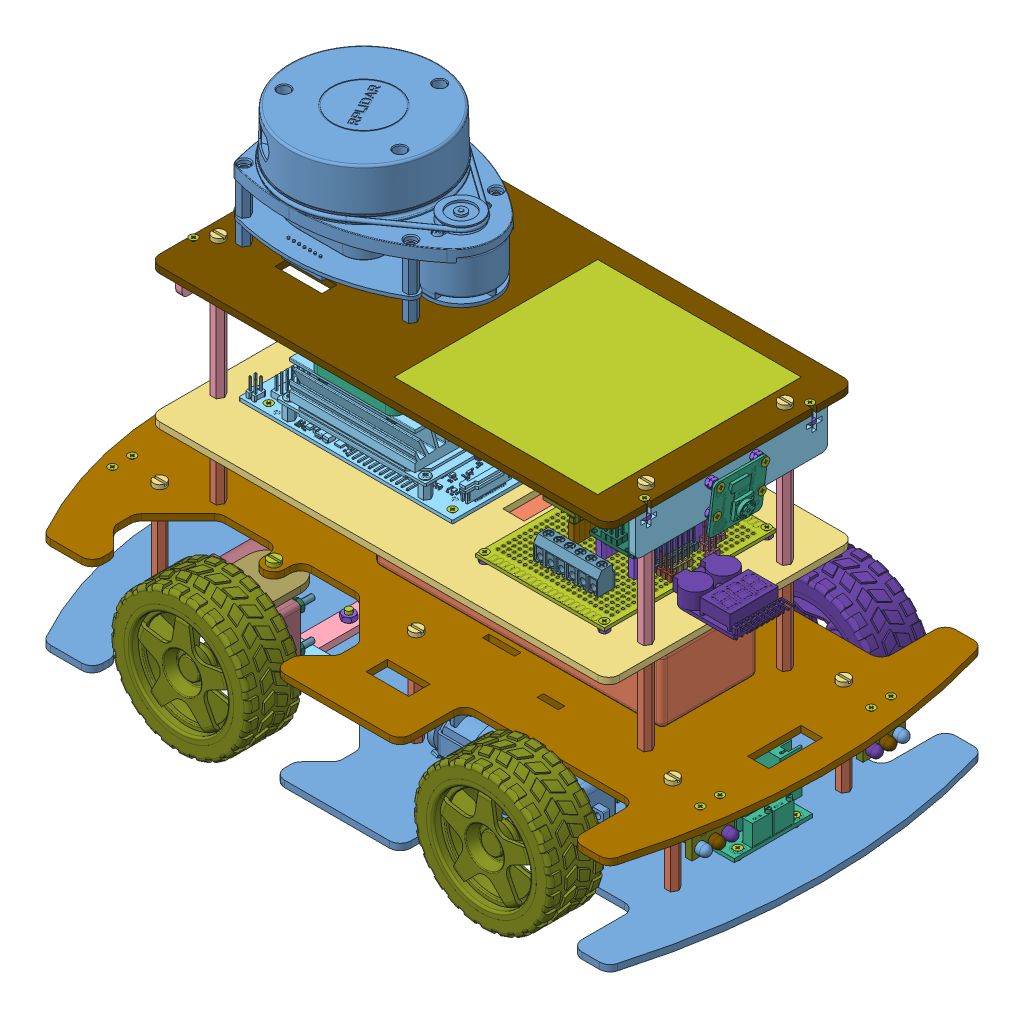
SolidWorks assembly Nigel - Motion Analysis, configuration Default. Lengths in mm.
Overall size (300 217.1 179.17).
273 component instances, 61 part files, 576 mates.
Components (placement in the parent):
- Platform 1-1: Platform 1 [Default] at origin size (300 3 175)
- M3x40 F-F Standoff-1: M3x40 F-F Standoff [Default] at (-1.4467 -726.2923 -120.9176) size (5.77 40 5)
- M3x40 F-F Standoff-2: M3x40 F-F Standoff [Default] at (-1.4467 -726.2923 -200.9176) size (5.77 40 5)
- M3x40 F-F Standoff-3: M3x40 F-F Standoff [Default] at (118.5533 -726.2923 -120.9176) size (5.77 40 5)
- M3x40 F-F Standoff-4: M3x40 F-F Standoff [Default] at (118.5533 -726.2923 -200.9176) size (5.77 40 5)
- M3x40 F-F Standoff-5: M3x40 F-F Standoff [Default] at (238.5533 -726.2923 -120.9176) size (5.77 40 5)
- M3x40 F-F Standoff-6: M3x40 F-F Standoff [Default] at (238.5533 -726.2923 -200.9176) size (5.77 40 5)
- M3x8 Bolt-1: M3x8 Bolt [Default] at (-120 0 40) x (1 0 0) z (0 0 -1) size (5.7 10 5.7)
- M3x8 Bolt-2: M3x8 Bolt [Default] at (-120 0 -40) x (1 0 0) z (0 0 -1) size (5.7 10 5.7)
- M3x8 Bolt-3: M3x8 Bolt [Default] at (0 0 40) x (1 0 0) z (0 0 -1) size (5.7 10 5.7)
- M3x8 Bolt-4: M3x8 Bolt [Default] at (0 0 -40) x (1 0 0) z (0 0 -1) size (5.7 10 5.7)
- M3x8 Bolt-5: M3x8 Bolt [Default] at (120 0 40) x (1 0 0) z (0 0 -1) size (5.7 10 5.7)
- M3x8 Bolt-6: M3x8 Bolt [Default] at (120 0 -40) x (1 0 0) z (0 0 -1) size (5.7 10 5.7)
- Steering Link 1-2: Steering Link 1 [Default] at (-61.537 3 0) x (0 0 1) z (-1 0 0) size (100 3 10)
- Steering Knuckle 1-1: Steering Knuckle 1 [Default] at (-61.537 6 0) x (0 0 -1) z (1 0 0) size (32.95 3 42.5)
- Steering Knuckle 1-2: Steering Knuckle 1 [Default] at (-61.537 9 0) x (0 0 1) z (1 0 0) size (32.95 3 42.5)
- Steering Link 2-2: Steering Link 2 [Default] at (-11.537 9 0) x (0 0 1) z (-1 0 0) size (84.1 3 10)
- M3x10 Bolt-1: M3x10 Bolt [Default] at (-61.537 0 -10) x (1 0 0) z (0 0 -1) size (5.7 12 5.7)
- M3 Nut-2: M3 Nut [Default] at (-61.537 6 -10) size (5.5 2.4 6.98)
- M3x10 Bolt-2: M3x10 Bolt [Default] at (-61.537 0 10) x (1 0 0) z (0 0 -1) size (5.7 12 5.7)
- M3 Nut-3: M3 Nut [Default] at (-61.537 6 10) size (5.5 2.4 6.98)
- M3x14 Bolt-1: M3x14 Bolt [Default] at (-61.537 9 45) size (5.7 16 5.7)
- M3 Nut-4: M3 Nut [Default] at (-61.537 -2.6 45) size (5.5 2.4 6.98)
- M3x14 Bolt-2: M3x14 Bolt [Default] at (-61.537 9 -45) size (5.7 16 5.7)
- M3 Nut-5: M3 Nut [Default] at (-61.537 -2.6 -45) size (5.5 2.4 6.98)
- M3x10 Bolt-3: M3x10 Bolt [Default] at (-36.537 5.8 37.0517) x (1 0 0) z (0 0 -1) size (5.7 12 5.7)
- M3 Nut-6: M3 Nut [Default] at (-36.537 12 37.0517) size (5.5 2.4 6.98)
- M3x10 Bolt-4: M3x10 Bolt [Default] at (-36.537 5.8 -37.0517) x (1 0 0) z (0 0 -1) size (5.7 12 5.7)
- M3 Nut-7: M3 Nut [Default] at (-36.537 12 -37.0517) size (5.5 2.4 6.98)
- M3x25 Bolt-1: M3x25 Bolt [Default] at (-36.537 9 0) x (1 0 0) z (0 0 -1) size (5.7 27 5.7)
- M3 Nut-1: M3 Nut [Default] at (-36.537 12 0) size (5.5 2.4 6.98)
- M3 Nut-14: M3 Nut [Default] at (-36.537 25.75 0) size (5.5 2.4 6.98)
- Front Motor Mount-1: Front Motor Mount [Default] at (-61.537 23 -60.5) x (1 0 0) z (0 0 -1) size (25 37 3)
- Front Motor Mount-2: Front Motor Mount [Default] at (-61.537 23 57.5) x (1 0 0) z (0 0 -1) size (25 37 3)
- Steering Knuckle 2-1: Steering Knuckle 2 [Default] at (-61.537 40 50) x (0 0 -1) z (1 0 0) size (30 3 25)
- Steering Knuckle 2-2: Steering Knuckle 2 [Default] at (-61.537 40 -50) x (0 0 1) z (-1 0 0) size (30 3 25)
- Front Wheel Hub-1: Front Wheel Hub [Default] at (-71.9938 11.75 35.7704) x (0 0 -1) z (1 0 0) size (40.5 22.5 47)
- M2.5x25 Bolt-1: M2.5x25 Bolt [Default] at (-53.037 31.75 60.5) x (1 0 0) z (0 -1 0) size (5.1 27 5.1)
- M2.5 Nut-1: M2.5 Nut [Default] at (-53.037 31.75 41.5) x (1 0 0) z (0 -1 0) size (5 2 6.35)
- M2.5x25 Bolt-2: M2.5x25 Bolt [Default] at (-53.037 14.25 60.5) x (1 0 0) z (0 -1 0) size (5.1 27 5.1)
- M2.5 Nut-2: M2.5 Nut [Default] at (-53.037 14.25 41.5) x (1 0 0) z (0 -1 0) size (5 2 6.35)
- Front Wheel Hub-2: Front Wheel Hub [Default] at (-71.9938 34.25 -35.7704) x (0 0 1) z (1 0 0) size (40.5 22.5 47)
- M2.5x25 Bolt-3: M2.5x25 Bolt [Default] at (-53.037 31.75 -60.5) x (1 0 0) z (0 1 0) size (5.1 27 5.1)
- M2.5 Nut-3: M2.5 Nut [Default] at (-53.037 31.75 -43.5) x (1 0 0) z (0 -1 0) size (5 2 6.35)
- M2.5x25 Bolt-4: M2.5x25 Bolt [Default] at (-53.037 14.25 -60.5) x (1 0 0) z (0 1 0) size (5.1 27 5.1)
- M2.5 Nut-4: M2.5 Nut [Default] at (-53.037 14.25 -43.5) x (1 0 0) z (0 -1 0) size (5 2 6.35)
- Left Wheel-1: Left Wheel [Default] at (-79.9477 -3.5128 34.4259) size (65 65 30.09)
- Right Wheel-1: Right Wheel [Default] at (-48.2819 2.8225 -42.4013) x (-1 0 0) z (0 0 -1) size (65 65 30.09)
- Rear Motor Mount-1: Rear Motor Mount [Default] at (59.4 23 -37.9) size (25 46 3)
- Rear Motor Mount-2: Rear Motor Mount [Default] at (59.4 23 34.9) size (25 46 3)
- Rear Motor-1: Rear Motor [Default] at (119.5998 48.0831 -84.1205) x (0 -1 0) z (-1 0 0) size (29.86 44.39 75.48)
- Rear Motor-2: Rear Motor [Default] at (119.5998 -2.0831 84.1205) x (0 1 0) z (-1 0 0) size (29.86 44.39 75.48)
- M3x25 Bolt-2: M3x25 Bolt [Default] at (59.4 31.75 56.5) x (1 0 0) z (0 -1 0) size (5.7 27 5.7)
- M3 Nut-10: M3 Nut [Default] at (59.4 31.75 32.5) x (1 0 0) z (0 -1 0) size (5.5 2.4 6.98)
- M3x25 Bolt-3: M3x25 Bolt [Default] at (59.4 14.25 56.5) x (1 0 0) z (0 -1 0) size (5.7 27 5.7)
- M3 Nut-11: M3 Nut [Default] at (59.4 14.25 32.5) x (1 0 0) z (0 -1 0) size (5.5 2.4 6.98)
- M3x25 Bolt-4: M3x25 Bolt [Default] at (59.4 31.75 -56.5) x (1 0 0) z (0 1 0) size (5.7 27 5.7)
- M3 Nut-12: M3 Nut [Default] at (59.4 31.75 -34.9) x (1 0 0) z (0 -1 0) size (5.5 2.4 6.98)
- M3x25 Bolt-5: M3x25 Bolt [Default] at (59.4 14.25 -56.5) x (1 0 0) z (0 1 0) size (5.7 27 5.7)
- M3 Nut-13: M3 Nut [Default] at (59.4 14.25 -34.9) x (1 0 0) z (0 -1 0) size (5.5 2.4 6.98)
- Left Wheel-2: Left Wheel [Default] at (61.5893 -3.6128 34.4259) size (65 65 30.09)
- Right Wheel-2: Right Wheel [Default] at (93.2551 2.9225 -42.4013) x (-1 0 0) z (0 0 -1) size (65 65 30.09)
- Motor Driver-1: Motor Driver [Default] at (32.2636 -15.779 -17.5479) x (0 0 1) z (-1 0 0) size (49.64 15.8 28)
- M4x5 Spacer-1: M4x5 Spacer [Default] at (-15 3 21) size (7 5 7)
- M4x5 Spacer-2: M4x5 Spacer [Default] at (-15 3 -21) size (7 5 7)
- M4x5 Spacer-3: M4x5 Spacer [Default] at (9 3 21) size (7 5 7)
- M4x5 Spacer-4: M4x5 Spacer [Default] at (9 3 -21) size (7 5 7)
- M3x14 Bolt-3: M3x14 Bolt [Default] at (-15 9.5 21) size (5.7 16 5.7)
- M3 Nut-15: M3 Nut [Default] at (-15 -2.4 21) size (5.5 2.4 6.98)
- M3x14 Bolt-4: M3x14 Bolt [Default] at (-15 9.5 -21) size (5.7 16 5.7)
- M3 Nut-16: M3 Nut [Default] at (-15 -2.4 -21) size (5.5 2.4 6.98)
- M3x14 Bolt-5: M3x14 Bolt [Default] at (9 9.5 21) size (5.7 16 5.7)
- M3 Nut-17: M3 Nut [Default] at (9 -2.4 21) size (5.5 2.4 6.98)
- M3x14 Bolt-6: M3x14 Bolt [Default] at (9 9.5 -21) size (5.7 16 5.7)
- M3 Nut-18: M3 Nut [Default] at (9 -2.4 -21) size (5.5 2.4 6.98)
- M12 Push Button-1: M12 Push Button [Default] at (36 0 0) x (1 0 0) z (0 -1 0) size (15.74 16.08 24.73)
- M12 Push Button Nut-1: M12 Push Button Nut [Default] at (36 -0.5 0) x (1 0 0) z (0 -1 0) size (15.79 14.76 2.3)
- Buck Converter-2: Buck Converter [Default] at (94.4 5.5 0) size (65.3 28.6 46.4)
- M2x10 Bolt-5: M2x10 Bolt [Default] at (65 7.56 13.4) size (3.8 10 3.8)
- M2 Nut-5: M2 Nut [Default] at (65 -1.6 13.4) size (4 1.6 5.08)
- M2x10 Bolt-6: M2x10 Bolt [Default] at (65 7.56 -13.4) size (3.8 10 3.8)
- M2 Nut-6: M2 Nut [Default] at (65 -1.6 -13.4) size (4 1.6 5.08)
- M2x10 Bolt-7: M2x10 Bolt [Default] at (123.8 7.56 13.4) size (3.8 10 3.8)
- M2 Nut-7: M2 Nut [Default] at (123.8 -1.6 13.4) size (4 1.6 5.08)
- M2x10 Bolt-8: M2x10 Bolt [Default] at (123.8 7.56 -13.4) size (3.8 10 3.8)
- M2 Nut-8: M2 Nut [Default] at (123.8 -1.6 -13.4) size (4 1.6 5.08)
- Platform 2-1: Platform 2 [Default] at (0 43 0) size (300 3 175)
- M3x8 Bolt-7: M3x8 Bolt [Default] at (-120 46 40) size (5.7 10 5.7)
- M3x8 Bolt-8: M3x8 Bolt [Default] at (-120 46 -40) size (5.7 10 5.7)
- M3x8 Bolt-9: M3x8 Bolt [Default] at (0 46 40) size (5.7 10 5.7)
- M3x8 Bolt-10: M3x8 Bolt [Default] at (0 46 -40) size (5.7 10 5.7)
- M3x8 Bolt-11: M3x8 Bolt [Default] at (120 46 40) size (5.7 10 5.7)
- M3x8 Bolt-12: M3x8 Bolt [Default] at (120 46 -40) size (5.7 10 5.7)
- M3x10 Bolt-5: M3x10 Bolt [Default] at (-61.537 46 45) size (5.7 12 5.7)
- M3 Nut-8: M3 Nut [Default] at (-61.537 37.4 45) size (5.5 2.4 6.98)
- M3x10 Bolt-6: M3x10 Bolt [Default] at (-61.537 46 -45) size (5.7 12 5.7)
- M3 Nut-9: M3 Nut [Default] at (-61.537 37.4 -45) size (5.5 2.4 6.98)
- M3x40 F-F Standoff-7: M3x40 F-F Standoff [Default] at (18.5533 -683.2923 -128.4176) size (5.77 40 5)
- M3x40 F-F Standoff-8: M3x40 F-F Standoff [Default] at (18.5533 -683.2923 -193.4176) size (5.77 40 5)
- M3x40 F-F Standoff-9: M3x40 F-F Standoff [Default] at (218.5533 -683.2923 -128.4176) size (5.77 40 5)
- M3x40 F-F Standoff-10: M3x40 F-F Standoff [Default] at (218.5533 -683.2923 -193.4176) size (5.77 40 5)
- M3x8 Bolt-13: M3x8 Bolt [Default] at (-100 43 32.5) x (1 0 0) z (0 0 -1) size (5.7 10 5.7)
- M3x8 Bolt-14: M3x8 Bolt [Default] at (-100 43 -32.5) x (1 0 0) z (0 0 -1) size (5.7 10 5.7)
- M3x8 Bolt-15: M3x8 Bolt [Default] at (100 43 32.5) x (1 0 0) z (0 0 -1) size (5.7 10 5.7)
- M3x8 Bolt-16: M3x8 Bolt [Default] at (100 43 -32.5) x (1 0 0) z (0 0 -1) size (5.7 10 5.7)
- MG996R Servo Motor-1: MG996R Servo Motor [Default] at (-69.1359 43 0) x (1 0 0) z (0 0 -1) size (56.95 44.55 19.7)
- M4x10 Bolt-1: M4x10 Bolt [Default] at (-93.847 46 4.925) size (7.4 12.2 7.4)
- M4 Nut-1: M4 Nut [Default] at (-93.847 37.4 4.925) size (7 3.2 8.89)
- M4x10 Bolt-2: M4x10 Bolt [Default] at (-93.847 46 -4.925) size (7.4 12.2 7.4)
- M4 Nut-2: M4 Nut [Default] at (-93.847 37.4 -4.925) size (7 3.2 8.89)
- M4x10 Bolt-3: M4x10 Bolt [Default] at (-43.327 46 4.925) size (7.4 12.2 7.4)
- M4 Nut-3: M4 Nut [Default] at (-43.327 37.4 4.925) size (7 3.2 8.89)
- M4x10 Bolt-4: M4x10 Bolt [Default] at (-43.327 46 -4.925) size (7.4 12.2 7.4)
- M4 Nut-4: M4 Nut [Default] at (-43.327 37.4 -4.925) size (7 3.2 8.89)
- MG996R Servo Horn-1: MG996R Servo Horn [Default] at (-59.0359 25.75 0) x (0 0 -1) z (1 0 0) size (20 4.5 20)
- M3x6 Bolt-1: M3x6 Bolt [Default] at (-59.0359 25.75 0) x (1 0 0) z (0 0 -1) size (5.6 7.65 5.6)
- Acrylic Servo Horn-1: Acrylic Servo Horn [Default] at (-59.0359 22.75 0) x (0 0 1) z (-1 0 0) size (20 3 40)
- M3x6 Bolt-2: M3x6 Bolt [Default] at (-66.0359 22.75 0) x (1 0 0) z (0 0 -1) size (5.6 7.65 5.6)
- M3x6 Bolt-3: M3x6 Bolt [Default] at (-59.0359 22.75 7) x (1 0 0) z (0 0 -1) size (5.6 7.65 5.6)
- M3x6 Bolt-4: M3x6 Bolt [Default] at (-52.0359 22.75 0) x (1 0 0) z (0 0 -1) size (5.6 7.65 5.6)
- M3x6 Bolt-5: M3x6 Bolt [Default] at (-59.0359 22.75 -7) x (1 0 0) z (0 0 -1) size (5.6 7.65 5.6)
- LED Mount-1: LED Mount [Default] at (-139 35.5 40) x (0 0 -1) z (1 0 0) size (20 15 3)
- M2x10 Bolt-9: M2x10 Bolt [Default] at (-137.5 46.8 44.6) size (3.8 10 3.8)
- M2 Nut-9: M2 Nut [Default] at (-137.5 38.9 44.6) size (4 1.6 5.08)
- M2x10 Bolt-10: M2x10 Bolt [Default] at (-137.5 46.8 35.4) size (3.8 10 3.8)
- M2 Nut-10: M2 Nut [Default] at (-137.5 38.9 35.4) size (4 1.6 5.08)
- LED Mount-2: LED Mount [Default] at (-139 35.5 -40) x (0 0 -1) z (1 0 0) size (20 15 3)
- M2x10 Bolt-11: M2x10 Bolt [Default] at (-137.5 46.8 -35.4) size (3.8 10 3.8)
- M2 Nut-11: M2 Nut [Default] at (-137.5 38.9 -35.4) size (4 1.6 5.08)
- M2x10 Bolt-12: M2x10 Bolt [Default] at (-137.5 46.8 -44.6) size (3.8 10 3.8)
- M2 Nut-12: M2 Nut [Default] at (-137.5 38.9 -44.6) size (4 1.6 5.08)
- LED Mount-3: LED Mount [Default] at (136 35.5 40) x (0 0 -1) z (1 0 0) size (20 15 3)
- M2x10 Bolt-13: M2x10 Bolt [Default] at (137.5 46.8 44.6) size (3.8 10 3.8)
- M2 Nut-13: M2 Nut [Default] at (137.5 38.9 44.6) size (4 1.6 5.08)
- M2x10 Bolt-14: M2x10 Bolt [Default] at (137.5 46.8 35.4) size (3.8 10 3.8)
- M2 Nut-14: M2 Nut [Default] at (137.5 38.9 35.4) size (4 1.6 5.08)
- LED Mount-4: LED Mount [Default] at (136 35.5 -40) x (0 0 -1) z (1 0 0) size (20 15 3)
- M2x10 Bolt-15: M2x10 Bolt [Default] at (137.5 46.8 -35.4) size (3.8 10 3.8)
- M2 Nut-15: M2 Nut [Default] at (137.5 38.9 -35.4) size (4 1.6 5.08)
- M2x10 Bolt-16: M2x10 Bolt [Default] at (137.5 46.8 -44.6) size (3.8 10 3.8)
- M2 Nut-16: M2 Nut [Default] at (137.5 38.9 -44.6) size (4 1.6 5.08)
- 5mm White LED-1: 5mm White LED [Valor predeterminado] at (-135 31.75 33.75) x (0 0 1) z (-1 0 0) size (5.5 6 15.8)
- 5mm White LED-2: 5mm White LED [Valor predeterminado] at (-135 31.75 -33.75) x (0 0 -1) z (-1 0 0) size (5.5 6 15.8)
- 5mm White LED-3: 5mm White LED [Valor predeterminado] at (-135 31.75 40) x (0 0 1) z (-1 0 0) size (5.5 6 15.8)
- 5mm White LED-4: 5mm White LED [Valor predeterminado] at (-135 31.75 -40) x (0 0 -1) z (-1 0 0) size (5.5 6 15.8)
- 5mm White LED-5: 5mm White LED [Valor predeterminado] at (135 31.75 33.75) x (0 0 -1) z (1 0 0) size (5.5 6 15.8)
- 5mm White LED-6: 5mm White LED [Valor predeterminado] at (135 31.75 -33.75) x (0 0 1) z (1 0 0) size (5.5 6 15.8)
- 5mm Red LED-1: 5mm Red LED [Valor predeterminado] at (135 31.75 40) x (0 0 -1) z (1 0 0) size (5.5 6 15.8)
- 5mm Red LED-2: 5mm Red LED [Valor predeterminado] at (135 31.75 -40) x (0 0 1) z (1 0 0) size (5.5 6 15.8)
- 5mm Amber LED-1: 5mm Amber LED [Valor predeterminado] at (-135 31.75 46.25) x (0 0 1) z (-1 0 0) size (5.5 6 15.8)
- 5mm Amber LED-2: 5mm Amber LED [Valor predeterminado] at (-135 31.75 -46.25) x (0 0 -1) z (-1 0 0) size (5.5 6 15.8)
- 5mm Amber LED-3: 5mm Amber LED [Valor predeterminado] at (135 31.75 46.25) x (0 0 -1) z (1 0 0) size (5.5 6 15.8)
- 5mm Amber LED-4: 5mm Amber LED [Valor predeterminado] at (135 31.75 -46.25) x (0 0 1) z (1 0 0) size (5.5 6 15.8)
- 11.1V 5200mAh LiPo Battery-1: 11.1V 5200mAh LiPo Battery [Default] at (30 46 0) size (135 31 45)
- Platform 3-1: Platform 3 [Default] at (0 86 0) size (215 3 115)
- M3x60 M-F Standoff-1: M3x60 M-F Standoff [Default] at (18.5533 -640.2923 -128.4176) size (5.77 66 5)
- M3x60 M-F Standoff-2: M3x60 M-F Standoff [Default] at (18.5533 -640.2923 -193.4176) size (5.77 66 5)
- M3x60 M-F Standoff-3: M3x60 M-F Standoff [Default] at (218.5533 -640.2923 -128.4176) size (5.77 66 5)
- M3x60 M-F Standoff-4: M3x60 M-F Standoff [Default] at (218.5533 -640.2923 -193.4176) size (5.77 66 5)
- Jetson Nano B01-1: Jetson Nano B01 [Default] at (6 91.5 -29) x (-1 0 0) z (0 1 0) size (100 81.03 30.51)
- M2x10 Bolt-17: M2x10 Bolt [Default] at (-80 93.595 29) size (3.8 10 3.8)
- M2 Nut-17: M2 Nut [Default] at (-80 84.4 29) size (4 1.6 5.08)
- M2x10 Bolt-18: M2x10 Bolt [Default] at (-80 93.595 -29) size (3.8 10 3.8)
- M2 Nut-18: M2 Nut [Default] at (-80 84.4 -29) size (4 1.6 5.08)
- M2x10 Bolt-19: M2x10 Bolt [Default] at (6 93.595 29) size (3.8 10 3.8)
- M2 Nut-19: M2 Nut [Default] at (6 84.4 29) size (4 1.6 5.08)
- M2x10 Bolt-20: M2x10 Bolt [Default] at (6 93.595 -29) size (3.8 10 3.8)
- M2 Nut-20: M2 Nut [Default] at (6 84.4 -29) size (4 1.6 5.08)
- 4020 DC Fan-1: 4020 DC Fan [Default] at (-38 129.7762 12.3) x (1 0 0) z (0 -1 0) size (40.27 40.57 21)
- M2.5x25 Bolt-5: M2.5x25 Bolt [Default] at (-54 139.7762 28.3) size (5.1 27 5.1)
- M2.5 Nut-5: M2.5 Nut [Default] at (-54 116.2762 28.3) size (5 2 6.35)
- M2.5x25 Bolt-6: M2.5x25 Bolt [Default] at (-22 139.7762 28.3) size (5.1 27 5.1)
- M2.5 Nut-6: M2.5 Nut [Default] at (-22 116.2762 28.3) size (5 2 6.35)
- M2.5x25 Bolt-7: M2.5x25 Bolt [Default] at (-54 139.7762 -3.7) size (5.1 27 5.1)
- M2.5 Nut-7: M2.5 Nut [Default] at (-54 116.2762 -3.7) size (5 2 6.35)
- M2.5x25 Bolt-8: M2.5x25 Bolt [Default] at (-22 139.7762 -3.7) size (5.1 27 5.1)
- M2.5 Nut-8: M2.5 Nut [Default] at (-22 116.2762 -3.7) size (5 2 6.35)
- Auxillary Board-1: Auxillary Board [Default] at (58 90.6 0) x (0 0 -1) z (1 0 0) size (80.2 24 60.2)
  - PCB-1: PCB [Default] at origin size (80.2 1.52 60.2)
  - Female Pin Header 1x15-1: Female Pin Header 1x15 [Default] at (-12.705 1.5 16.51) x (1 0 0) z (0 1 0) size (38.1 2.54 11.7)
  - Female Pin Header 1x15-2: Female Pin Header 1x15 [Default] at (-12.705 1.5 1.27) x (1 0 0) z (0 1 0) size (38.1 2.54 11.7)
  - Female Pin Header 1x10-1: Female Pin Header 1x10 [Default] at (-12.705 1.5 -11.43) x (1 0 0) z (0 1 0) size (25.4 2.54 11.7)
  - Male Pin Header 1x8-1: Male Pin Header 1x8 [Default] at (-5.075 1.4986 19.05) x (1 0 0) z (0 1 0) size (20.33 2.55 12.7)
  - Male Pin Header 1x3-1: Male Pin Header 1x3 [Default] at (-5.075 1.4986 26.67) x (0 0 -1) z (0 1 0) size (7.63 2.55 12.7)
  - Male Pin Header 1x4-1: Male Pin Header 1x4 [Default] at (-2.535 1.4986 24.13) x (1 0 0) z (0 1 0) size (10.17 2.55 12.7)
  - Male Pin Header 1x2-1: Male Pin Header 1x2 [Default] at (15.245 1.4986 24.13) x (0 0 -1) z (0 1 0) size (5.09 2.55 12.7)
  - Male Pin Header 1x2-2: Male Pin Header 1x2 [Default] at (12.705 1.4986 26.67) x (1 0 0) z (0 1 0) size (5.09 2.55 12.7)
  - Male Pin Header 1x2-3: Male Pin Header 1x2 [Default] at (17.785 1.4986 21.59) x (0 0 -1) z (0 1 0) size (5.09 2.55 12.7)
  - Male Pin Header 1x2-4: Male Pin Header 1x2 [Default] at (20.325 1.4986 21.59) x (0 0 -1) z (0 1 0) size (5.09 2.55 12.7)
  - Male Pin Header 1x2-5: Male Pin Header 1x2 [Default] at (22.865 1.4986 21.59) x (0 0 -1) z (0 1 0) size (5.09 2.55 12.7)
  - Male Pin Header 1x2-6: Male Pin Header 1x2 [Default] at (22.865 1.4986 -1.27) x (0 0 -1) z (0 1 0) size (5.09 2.55 12.7)
  - Male Pin Header 1x2-7: Male Pin Header 1x2 [Default] at (15.245 1.4986 -1.27) x (0 0 -1) z (0 1 0) size (5.09 2.55 12.7)
  - Male Pin Header 1x2-8: Male Pin Header 1x2 [Default] at (12.705 1.4986 -1.27) x (0 0 -1) z (0 1 0) size (5.09 2.55 12.7)
  - Screw Terminal Block-1: Screw Terminal Block [Default] at (-25.4 1.5 1.27) x (0 0 1) z (-1 0 0) size (30.15 12 8)
  - Arduino Nano V3-1: Arduino Nano V3 [Default] at (-16.775 14.1 17.78) x (1 0 0) z (0 0 -1) size (45.1 18 17.9)
  - MPU-9250-1: MPU-9250 [Default] at (11.225 14.3786 -9.93) x (0 0 1) z (-1 0 0) size (15 12.78 25.4)
- M2 Nut-47: M2 Nut [Default] at (30 89 38) size (4 1.6 5.08)
- M2 Nut-48: M2 Nut [Default] at (30 89 -38) size (4 1.6 5.08)
- M2 Nut-49: M2 Nut [Default] at (86 89 38) size (4 1.6 5.08)
- M2 Nut-50: M2 Nut [Default] at (86 89 -38) size (4 1.6 5.08)
- M2x10 Bolt-37: M2x10 Bolt [Default] at (30 92.85 38) size (3.8 10 3.8)
- M2 Nut-37: M2 Nut [Default] at (30 84.4 38) size (4 1.6 5.08)
- M2x10 Bolt-38: M2x10 Bolt [Default] at (30 92.85 -38) size (3.8 10 3.8)
- M2 Nut-38: M2 Nut [Default] at (30 84.4 -38) size (4 1.6 5.08)
- M2x10 Bolt-39: M2x10 Bolt [Default] at (86 92.85 38) size (3.8 10 3.8)
- M2 Nut-39: M2 Nut [Default] at (86 84.4 38) size (4 1.6 5.08)
- M2x10 Bolt-40: M2x10 Bolt [Default] at (86 92.85 -38) size (3.8 10 3.8)
- M2 Nut-40: M2 Nut [Default] at (86 84.4 -38) size (4 1.6 5.08)
- LiPo Battery Voltage Tester-1: LiPo Battery Voltage Tester [Default] at (105.6 89.5 0) x (0 0 -1) z (1 0 0) size (25 10.5 37.93)
- Platform 4-1: Platform 4 [Default] at (0 149 0) size (215 3 115)
- M3x8 Bolt-17: M3x8 Bolt [Default] at (-100 152 32.5) size (5.7 10 5.7)
- M3x8 Bolt-18: M3x8 Bolt [Default] at (-100 152 -32.5) size (5.7 10 5.7)
- M3x8 Bolt-19: M3x8 Bolt [Default] at (100 152 32.5) size (5.7 10 5.7)
- M3x8 Bolt-20: M3x8 Bolt [Default] at (100 152 -32.5) size (5.7 10 5.7)
- RPLIDAR A1-1: RPLIDAR A1 [Default] at (26.0533 -565.6923 -132.9176) size (101.56 55.5 71.81)
- M2.5x8 Bolt-1: M2.5x8 Bolt [Default] at (-92.5 148 28) x (1 0 0) z (0 0 -1) size (4.7 8 4.7)
- M2.5x8 Bolt-2: M2.5x8 Bolt [Default] at (-92.5 148 -28) x (1 0 0) z (0 0 -1) size (4.7 8 4.7)
- M2.5x8 Bolt-3: M2.5x8 Bolt [Default] at (-22.5 148 20) x (1 0 0) z (0 0 -1) size (4.7 8 4.7)
- M2.5x8 Bolt-4: M2.5x8 Bolt [Default] at (-22.5 148 -20) x (1 0 0) z (0 0 -1) size (4.7 8 4.7)
- RPLIDAR Adapter-1: RPLIDAR Adapter [Default] at (-64.5 147.4 -34) x (0 0 1) z (1 0 0) size (40 6.5 20)
- M2 Nut-45: M2 Nut [Default] at (-57.5 147.4 -46.5) size (4 1.6 5.08)
- M2 Nut-46: M2 Nut [Default] at (-71.5 147.4 -46.5) size (4 1.6 5.08)
- M2 Nut-51: M2 Nut [Default] at (-57.5 147.4 -28) size (4 1.6 5.08)
- M2 Nut-52: M2 Nut [Default] at (-71.5 147.4 -28) size (4 1.6 5.08)
- M2x10 Bolt-21: M2x10 Bolt [Default] at (-57.5 145 -46.5) x (1 0 0) z (0 0 -1) size (3.8 10 3.8)
- M2 Nut-21: M2 Nut [Default] at (-57.5 152 -46.5) size (4 1.6 5.08)
- M2x10 Bolt-22: M2x10 Bolt [Default] at (-71.5 145 -46.5) x (1 0 0) z (0 0 -1) size (3.8 10 3.8)
- M2 Nut-22: M2 Nut [Default] at (-71.5 152 -46.5) size (4 1.6 5.08)
- M2x10 Bolt-23: M2x10 Bolt [Default] at (-57.5 145 -28) x (1 0 0) z (0 0 -1) size (3.8 10 3.8)
- M2 Nut-23: M2 Nut [Default] at (-57.5 152 -28) size (4 1.6 5.08)
- M2x10 Bolt-24: M2x10 Bolt [Default] at (-71.5 145 -28) x (1 0 0) z (0 0 -1) size (3.8 10 3.8)
- M2 Nut-24: M2 Nut [Default] at (-71.5 152 -28) size (4 1.6 5.08)
- Front Camera Mount-1: Front Camera Mount [Default] at (-107.5 140.25 0) x (0 0 -1) z (1 0 0) size (90 17.5 3)
- M2x10 Bolt-25: M2x10 Bolt [Default] at (-105.5 152.8 -38.7) size (3.8 10 3.8)
- M2 Nut-25: M2 Nut [Default] at (-105.5 144.9 -38.7) size (4 1.6 5.08)
- M2x10 Bolt-26: M2x10 Bolt [Default] at (-105.5 152.8 38.7) size (3.8 10 3.8)
- M2 Nut-26: M2 Nut [Default] at (-105.5 144.9 38.7) size (4 1.6 5.08)
- Rear Camera Mount-1: Rear Camera Mount [Default] at (104.5 140.25 0) x (0 0 -1) z (1 0 0) size (90 17.5 3)
- M2x10 Bolt-27: M2x10 Bolt [Default] at (105.5 152.8 38.7) size (3.8 10 3.8)
- M2 Nut-27: M2 Nut [Default] at (105.5 144.9 38.7) size (4 1.6 5.08)
- M2x10 Bolt-28: M2x10 Bolt [Default] at (105.5 152.8 -38.7) size (3.8 10 3.8)
- M2 Nut-28: M2 Nut [Default] at (105.5 144.9 -38.7) size (4 1.6 5.08)
- Raspberry Pi Camera V2.1-1: Raspberry Pi Camera V2.1 [Default] at (-109.6979 136.6712 0) x (-0.991907 -0.126964 0) z (0 0 -1) size (6.48 24.01 25.01)
- M2 Nut-53: M2 Nut [Default] at (-107.5 146.5 -10.5) x (0 1 0) z (0 0 1) size (4 1.6 5.08)
- M2 Nut-54: M2 Nut [Default] at (-107.5 146.5 10.5) x (0 1 0) z (0 0 1) size (4 1.6 5.08)
- M2 Nut-55: M2 Nut [Default] at (-107.5 134 -10.5) x (0 1 0) z (0 0 1) size (4 1.6 5.08)
- M2 Nut-56: M2 Nut [Default] at (-107.5 134 10.5) x (0 1 0) z (0 0 1) size (4 1.6 5.08)
- M2 Nut-57: M2 Nut [Default] at (-109.1 146.5 -10.5) x (0 1 0) z (0 0 1) size (4 1.6 5.08)
- M2 Nut-58: M2 Nut [Default] at (-109.1 146.5 10.5) x (0 1 0) z (0 0 1) size (4 1.6 5.08)
- M2x10 Bolt-29: M2x10 Bolt [Default] at (-113 146.5 -10.5) x (0 0 -1) z (0 1 0) size (3.8 10 3.8)
- M2 Nut-29: M2 Nut [Default] at (-104.5 146.5 -10.5) x (0 0 -1) z (0 -1 0) size (4 1.6 5.08)
- M2x10 Bolt-30: M2x10 Bolt [Default] at (-113 146.5 10.5) x (0 0 -1) z (0 1 0) size (3.8 10 3.8)
- M2 Nut-30: M2 Nut [Default] at (-104.5 146.5 10.5) x (0 0 -1) z (0 -1 0) size (4 1.6 5.08)
- M2x10 Bolt-31: M2x10 Bolt [Default] at (-111.4 134 -10.5) x (0 0 -1) z (0 1 0) size (3.8 10 3.8)
- M2 Nut-31: M2 Nut [Default] at (-104.5 134 -10.5) x (0 0 -1) z (0 -1 0) size (4 1.6 5.08)
- M2x10 Bolt-32: M2x10 Bolt [Default] at (-111.4 134 10.5) x (0 0 -1) z (0 1 0) size (3.8 10 3.8)
- M2 Nut-32: M2 Nut [Default] at (-104.5 134 10.5) x (0 0 -1) z (0 -1 0) size (4 1.6 5.08)
- Raspberry Pi Camera V2.1-2: Raspberry Pi Camera V2.1 [Default] at (109.6979 136.6712 0) x (0.991907 -0.126964 0) z (0 0 1) size (6.48 24.01 25.01)
- M2 Nut-59: M2 Nut [Default] at (109.1 146.5 10.5) x (0 1 0) z (0 0 1) size (4 1.6 5.08)
- M2 Nut-60: M2 Nut [Default] at (109.1 146.5 -10.5) x (0 1 0) z (0 0 1) size (4 1.6 5.08)
- M2 Nut-61: M2 Nut [Default] at (109.1 134 10.5) x (0 1 0) z (0 0 1) size (4 1.6 5.08)
- M2 Nut-62: M2 Nut [Default] at (109.1 134 -10.5) x (0 1 0) z (0 0 1) size (4 1.6 5.08)
- M2 Nut-63: M2 Nut [Default] at (110.7 146.5 10.5) x (0 1 0) z (0 0 1) size (4 1.6 5.08)
- M2 Nut-64: M2 Nut [Default] at (110.7 146.5 -10.5) x (0 1 0) z (0 0 1) size (4 1.6 5.08)
- M2x10 Bolt-33: M2x10 Bolt [Default] at (113 146.5 10.5) x (0 0 -1) z (0 -1 0) size (3.8 10 3.8)
- M2 Nut-33: M2 Nut [Default] at (102.9 146.5 10.5) x (0 0 -1) z (0 -1 0) size (4 1.6 5.08)
- M2x10 Bolt-34: M2x10 Bolt [Default] at (113 146.5 -10.5) x (0 0 -1) z (0 -1 0) size (3.8 10 3.8)
- M2 Nut-34: M2 Nut [Default] at (102.9 146.5 -10.5) x (0 0 -1) z (0 -1 0) size (4 1.6 5.08)
- M2x10 Bolt-35: M2x10 Bolt [Default] at (111.4 134 10.5) x (0 0 -1) z (0 -1 0) size (3.8 10 3.8)
- M2 Nut-35: M2 Nut [Default] at (102.9 134 10.5) x (0 0 -1) z (0 -1 0) size (4 1.6 5.08)
- M2x10 Bolt-36: M2x10 Bolt [Default] at (111.4 134 -10.5) x (0 0 -1) z (0 -1 0) size (3.8 10 3.8)
- M2 Nut-36: M2 Nut [Default] at (102.9 134 -10.5) x (0 0 -1) z (0 -1 0) size (4 1.6 5.08)
- AprilTag-1: AprilTag [Default] at (44.875 152 0) x (0 0 1) z (-1 0 0) size (95.25 0.06 95.25)
Mates (geometry in assembly coordinates):
- Coincident5: coincident: plane of Platform 1-1 through (-150 3 0) normal (0 1 0); plane of Steering Link 1-2 through (-61.537 3 -45) normal (0 -1 0)
- Concentric8: concentric: cylinder of Platform 1-1 through (-61.537 3 -45) axis (0 -1 0) radius 1.75; cylinder of Steering Link 1-2 through (-61.537 6 -45) axis (0 -1 0) radius 1.75
- Concentric11: concentric: cylinder of Platform 1-1 through (-61.537 3 45) axis (0 -1 0) radius 1.75; cylinder of Steering Link 1-2 through (-61.537 6 45) axis (0 -1 0) radius 1.75
- Coincident6: coincident: plane of Steering Knuckle 1-1 through (-36.537 6 37.0517) normal (0 -1 0); plane of Steering Link 1-2 through (-61.537 6 -45) normal (0 1 0)
- Concentric12: concentric: cylinder of Steering Knuckle 1-1 through (-61.537 9 45) axis (0 -1 0) radius 1.75; cylinder of Steering Link 1-2 through (-61.537 6 45) axis (0 -1 0) radius 1.75
- Coincident7: coincident: plane of Steering Knuckle 1-2 through (-36.537 6 -37.0517) normal (0 -1 0); plane of Steering Link 1-2 through (-61.537 6 -45) normal (0 1 0)
- Concentric13: concentric: cylinder of Steering Knuckle 1-2 through (-61.537 6 -45) axis (0 1 0) radius 1.75; cylinder of Steering Link 1-2 through (-61.537 6 -45) axis (0 -1 0) radius 1.75
- Coincident8: coincident: plane of Steering Knuckle 1-1 through (-36.537 9 37.0517) normal (0 1 0); plane of Steering Link 2-2 through (-36.537 9 -37.0517) normal (0 -1 0)
- Concentric14: concentric: cylinder of Steering Knuckle 1-1 through (-36.537 9 37.0517) axis (0 -1 0) radius 1.75; cylinder of Steering Link 2-2 through (-36.537 12 37.0517) axis (0 -1 0) radius 1.75
- Concentric15: concentric: cylinder of Steering Knuckle 1-2 through (-36.537 6 -37.0517) axis (0 1 0) radius 1.75; cylinder of Steering Link 2-2 through (-36.537 12 -37.0517) axis (0 -1 0) radius 1.75
- Coincident27: coincident: plane of Platform 1-1 through (-150 0 0) normal (0 -1 0); plane of Rear Motor Mount-1 through (54.4 0 -34.9) normal (0 -1 0)
- Coincident28: coincident: plane of Platform 1-1 through (64.4 3 -34.9) normal (-1 0 0); plane of Rear Motor Mount-1 through (64.4 0 -34.9) normal (1 0 0)
- Coincident29: coincident: plane of Platform 1-1 through (54.4 3 -37.9) normal (0 0 1); plane of Rear Motor Mount-1 through (59.4 23 -37.9) normal (0 0 -1)
- Coincident30: coincident: plane of Platform 1-1 through (-150 0 0) normal (0 -1 0); plane of Rear Motor Mount-2 through (54.4 0 37.9) normal (0 -1 0)
- Coincident31: coincident: plane of Platform 1-1 through (54.4 3 34.9) normal (1 0 0); plane of Rear Motor Mount-2 through (54.4 0 37.9) normal (-1 0 0)
- Coincident32: coincident: plane of Platform 1-1 through (54.4 3 37.9) normal (0 0 -1); plane of Rear Motor Mount-2 through (59.4 23 37.9) normal (0 0 1)
- Coincident33: coincident: plane of Rear Motor Mount-2 through (59.4 23 37.9) normal (0 0 1); plane of Rear Motor-2 through (54.2 11.75 37.9) normal (0 0 -1)
- Coincident35: coincident: plane of Rear Motor Mount-1 through (59.4 23 -37.9) normal (0 0 -1); plane of Rear Motor-1 through (54.2 34.25 -37.9) normal (0 0 1)
- Concentric46: concentric: cylinder of Front Wheel Hub-1 through (-53.037 31.75 58.5) axis (0 0 -1) radius 1.1; cylinder of Front Motor Mount-2 through (-53.037 31.75 60.5) axis (0 0 -1) radius 1.6
- Coincident51: coincident: plane of Front Wheel Hub-1 through (-92.537 34.25 57.5) normal (0 0 1); plane of Front Motor Mount-2 through (-61.537 23 57.5) normal (0 0 -1)
- Concentric48: concentric: cylinder of Front Wheel Hub-2 through (-53.037 31.75 -58.5) axis (0 0 1) radius 1.1; cylinder of Front Motor Mount-1 through (-53.037 31.75 -57.5) axis (0 0 -1) radius 1.6
- Coincident52: coincident: plane of Front Wheel Hub-2 through (-92.537 11.75 -57.5) normal (0 0 -1); plane of Front Motor Mount-1 through (-61.537 23 -57.5) normal (0 0 1)
- Coincident53: coincident: plane of Steering Knuckle 1-1 through (-66.537 9 60.5) normal (1 0 0); plane of Front Motor Mount-2 through (-66.537 9 60.5) normal (-1 0 0)
- Coincident54: coincident: plane of Steering Knuckle 1-1 through (-56.537 9 60.5) normal (0 0 -1); plane of Front Motor Mount-2 through (-61.537 23 60.5) normal (0 0 1)
- Coincident55: coincident: plane of Steering Knuckle 1-2 through (-56.537 6 -60.5) normal (0 0 1); plane of Front Motor Mount-1 through (-61.537 23 -60.5) normal (0 0 -1)
- Coincident58: coincident: plane of Steering Knuckle 1-2 through (-66.537 6 -60.5) normal (1 0 0); plane of Front Motor Mount-1 through (-66.537 9 -57.5) normal (-1 0 0)
- Coincident60: coincident: plane of Steering Knuckle 1-1 through (-36.537 6 37.0517) normal (0 -1 0); plane of Front Motor Mount-2 through (-66.537 6 60.5) normal (0 -1 0)
- Concentric51: concentric: cylinder of Front Wheel Hub-1 through (-53.037 14.25 58.5) axis (0 0 -1) radius 1.1; cylinder of Front Motor Mount-2 through (-53.037 14.25 60.5) axis (0 0 -1) radius 1.6
- Concentric52: concentric: cylinder of Front Wheel Hub-2 through (-53.037 14.25 -58.5) axis (0 0 1) radius 1.1; cylinder of Front Motor Mount-1 through (-53.037 14.25 -57.5) axis (0 0 -1) radius 1.6
- Coincident64: coincident: plane of Front Motor Mount-1 through (-66.537 40 -57.5) normal (-1 0 0); plane of Steering Knuckle 2-2 through (-66.537 43 -60.5) normal (1 0 0)
- Coincident65: coincident: plane of Front Motor Mount-2 through (-66.537 40 60.5) normal (-1 0 0); plane of Steering Knuckle 2-1 through (-66.537 43 60.5) normal (1 0 0)
- Concentric55: concentric: cylinder of Rear Motor Mount-2 through (59.4 31.75 37.9) axis (0 0 -1) radius 1.6; cylinder of Rear Motor-2 through (59.4 31.75 37.9) axis (0 0 1) radius 1.4
- Concentric56: concentric: cylinder of Rear Motor Mount-2 through (59.4 14.25 37.9) axis (0 0 -1) radius 1.6; cylinder of Rear Motor-2 through (59.4 14.25 37.9) axis (0 0 1) radius 1.4
- Concentric57: concentric: cylinder of Rear Motor Mount-1 through (59.4 31.75 -34.9) axis (0 0 -1) radius 1.6; cylinder of Rear Motor-1 through (59.4 31.75 -37.9) axis (0 0 -1) radius 1.4
- Concentric58: concentric: cylinder of Rear Motor Mount-1 through (59.4 14.25 -34.9) axis (0 0 -1) radius 1.6; cylinder of Rear Motor-1 through (59.4 14.25 -37.9) axis (0 0 -1) radius 1.4
- Coincident66: coincident: plane of Rear Motor Mount-1 through (54.4 43 -34.9) normal (-1 0 0); plane of Platform 2-1 through (54.4 46 -37.9) normal (1 0 0)
- Coincident67: coincident: plane of Rear Motor Mount-1 through (59.4 23 -37.9) normal (0 0 -1); plane of Platform 2-1 through (54.4 46 -37.9) normal (0 0 1)
- Coincident69: coincident: plane of Rear Motor Mount-1 through (54.4 46 -34.9) normal (0 1 0); plane of Platform 2-1 through (-150 46 0) normal (0 1 0)
- Coincident70: coincident: plane of Steering Knuckle 2-2 through (-71.537 43 -62.5) normal (0 1 0); plane of Platform 2-1 through (-150 43 0) normal (0 -1 0)
- Coincident71: coincident: plane of Steering Knuckle 2-1 through (-51.537 43 62.5) normal (0 1 0); plane of Platform 2-1 through (-150 43 0) normal (0 -1 0)
- Concentric59: concentric: cylinder of Steering Knuckle 2-1 through (-61.537 43 45) axis (0 -1 0) radius 1.75; cylinder of Platform 2-1 through (-61.537 46 45) axis (0 -1 0) radius 1.75
- Concentric60: concentric: cylinder of Steering Knuckle 2-2 through (-61.537 43 -45) axis (0 -1 0) radius 1.75; cylinder of Platform 2-1 through (-61.537 46 -45) axis (0 -1 0) radius 1.75
- Concentric61: concentric: cylinder of MG996R Servo Motor-1 through (-59.0359 71.3 0) axis (0 -1 0) radius 1.2; cylinder of MG996R Servo Horn-1 through (-59.0359 25.75 0) axis (0 1 0) radius 1.5
- Coincident72: coincident: plane of MG996R Servo Motor-1 through (-59.0359 26.75 0) normal (0 -1 0); plane of MG996R Servo Horn-1 through (-59.0359 26.75 0) normal (0 1 0)
- Concentric62: concentric: cylinder of Platform 2-1 through (-93.847 46 -4.925) axis (0 -1 0) radius 2.1; cylinder of MG996R Servo Motor-1 through (-93.847 40.6 -4.925) axis (0 1 0) radius 2.1
- Concentric63: concentric: cylinder of Platform 2-1 through (-93.847 46 4.925) axis (0 -1 0) radius 2.1; cylinder of MG996R Servo Motor-1 through (-93.847 40.6 4.925) axis (0 1 0) radius 2.1
- Coincident73: coincident: plane of Platform 2-1 through (-150 43 0) normal (0 -1 0); plane of MG996R Servo Motor-1 through (-95.8964 43 6.525) normal (0 1 0)
- Concentric64: concentric: cylinder of MG996R Servo Horn-1 through (-59.0359 25.75 0) axis (0 1 0) radius 1.5; cylinder of Acrylic Servo Horn-1 through (-59.0359 25.75 0) axis (0 -1 0) radius 3
- Concentric65: concentric: cylinder of MG996R Servo Horn-1 through (-66.0359 25.75 0) axis (0 1 0) radius 1.5; cylinder of Acrylic Servo Horn-1 through (-66.0359 25.75 0) axis (0 -1 0) radius 1.6
- Concentric66: concentric: cylinder of MG996R Servo Horn-1 through (-52.0359 25.75 0) axis (0 1 0) radius 1.5; cylinder of Acrylic Servo Horn-1 through (-52.0359 25.75 0) axis (0 -1 0) radius 1.6
- Coincident74: coincident: plane of MG996R Servo Horn-1 through (-59.0359 25.75 0) normal (0 -1 0); plane of Acrylic Servo Horn-1 through (-34.0359 25.75 0) normal (0 1 0)
- Coincident76: coincident: plane of Front Motor Mount-1 through (-66.537 43 -57.5) normal (0 1 0); plane of Steering Knuckle 2-2 through (-71.537 43 -62.5) normal (0 1 0)
- Concentric68: concentric: cylinder of Front Wheel Hub-1 through (-61.537 23 58.5) axis (0 0 -1) radius 3; cylinder of Left Wheel-1 through (-61.537 23 89.5) axis (0 0 1) radius 2.75
- Distance1: distance = 2 mm: plane of Left Wheel-1 through (-61.537 23 59.5) normal (0 0 -1); plane of Front Wheel Hub-1 through (-92.537 34.25 57.5) normal (0 0 1)
- Concentric69: concentric: cylinder of Front Wheel Hub-2 through (-61.537 23 -58.5) axis (0 0 1) radius 3; cylinder of Right Wheel-1 through (-61.537 23 -89.5) axis (0 0 -1) radius 2.75
- Distance2: distance = 2 mm: plane of Right Wheel-1 through (-61.537 23 -59.5) normal (0 0 1); plane of Front Wheel Hub-2 through (-92.537 11.75 -57.5) normal (0 0 -1)
- Concentric70: concentric: cylinder of Rear Motor-1 through (80 23.1 -65.5) axis (0 0 1) radius 2.5; cylinder of Right Wheel-2 through (80 23.1 -89.5) axis (0 0 -1) radius 2.75
- Distance3: distance = 3 mm: plane of Rear Motor-1 through (54.2 34.25 -56.5) normal (0 0 -1); plane of Right Wheel-2 through (80 23.1 -59.5) normal (0 0 1)
- Concentric71: concentric: cylinder of Rear Motor-2 through (80 22.9 65.5) axis (0 0 -1) radius 2.5; cylinder of Left Wheel-2 through (80 22.9 89.5) axis (0 0 1) radius 2.75
- Distance4: distance = 3 mm: plane of Left Wheel-2 through (80 22.9 59.5) normal (0 0 -1); plane of Rear Motor-2 through (54.2 11.75 56.5) normal (0 0 1)
- Concentric72: concentric: cylinder of Motor Driver-1 through (-15 9.5 21) axis (0 -1 0) radius 1.6; cylinder of Platform 1-1 through (-15 3 21) axis (0 -1 0) radius 1.6
- Concentric73: concentric: cylinder of Platform 1-1 through (-15 3 -21) axis (0 -1 0) radius 1.6; cylinder of Motor Driver-1 through (-15 9.5 -21) axis (0 -1 0) radius 1.6
- Parallel2: parallel: plane of Left Wheel-1 through (-60.987 23 89.5) normal (1 0 0); plane of Front Motor Mount-2 through (-49.037 9 60.5) normal (1 0 0)
- Parallel3: parallel: plane of Front Motor Mount-1 through (-49.037 9 -57.5) normal (1 0 0); plane of Right Wheel-1 through (-60.987 23 -89.5) normal (1 0 0)
- Parallel4: parallel: plane of Rear Motor Mount-2 through (71.9 43 37.9) normal (1 0 0); plane of Left Wheel-2 through (80.55 22.9 89.5) normal (1 0 0)
- Parallel5: parallel: plane of Rear Motor Mount-1 through (71.9 43 -34.9) normal (1 0 0); plane of Right Wheel-2 through (80.55 23.1 -89.5) normal (1 0 0)
- Coincident77: coincident: plane of Platform 2-1 through (-150 46 0) normal (0 1 0); plane of 11.1V 5200mAh LiPo Battery-1 through (30 46 0) normal (0 -1 0)
- Distance7: distance = 65 mm: plane of 11.1V 5200mAh LiPo Battery-1 through (-37.5 77 22.5) normal (0 0 1); plane of Platform 2-1 through (40 46 87.5) normal (0 0 1)
- Distance9: distance = 30 mm: plane of 11.1V 5200mAh LiPo Battery-1 through (97.5 77 22.5) normal (1 0 0); plane of Platform 2-1 through (127.5 46 12.5) normal (1 0 0)
- Coincident78: coincident: plane of Platform 2-1 through (-150 43 0) normal (0 -1 0); plane of LED Mount-1 through (-136 43 40) normal (0 1 0)
- Distance10: distance = 25 mm: plane of LED Mount-1 through (-136 35.5 30) normal (0 0 -1); plane of Platform 2-1 through (-127.5 46 5) normal (0 0 -1)
- Distance11: distance = 8.5 mm: plane of Platform 2-1 through (-127.5 46 5) normal (1 0 0); plane of LED Mount-1 through (-136 35.5 40) normal (1 0 0)
- Coincident81: coincident: plane of Platform 2-1 through (-150 43 0) normal (0 -1 0); plane of LED Mount-2 through (-136 43 -40) normal (0 1 0)
- Distance12: distance = 25 mm: plane of LED Mount-2 through (-136 35.5 -30) normal (0 0 1); plane of Platform 2-1 through (-127.5 46 -5) normal (0 0 1)
- Distance13: distance = 8.5 mm: plane of LED Mount-2 through (-136 35.5 -40) normal (1 0 0); plane of Platform 2-1 through (-127.5 46 5) normal (1 0 0)
- Coincident84: coincident: plane of Platform 2-1 through (-150 43 0) normal (0 -1 0); plane of LED Mount-3 through (139 43 40) normal (0 1 0)
- Distance14: distance = 17.5 mm: plane of LED Mount-3 through (139 35.5 30) normal (0 0 -1); plane of Platform 2-1 through (127.5 46 12.5) normal (0 0 -1)
- Distance15: distance = 1.5 mm: plane of Platform 2-1 through (137.5 46 12.5) normal (-1 0 0); plane of LED Mount-3 through (136 35.5 40) normal (-1 0 0)
- Coincident87: coincident: plane of Platform 2-1 through (-150 43 0) normal (0 -1 0); plane of LED Mount-4 through (139 43 -40) normal (0 1 0)
- Distance16: distance = 17.5 mm: plane of LED Mount-4 through (139 35.5 -30) normal (0 0 1); plane of Platform 2-1 through (127.5 46 -12.5) normal (0 0 1)
- Distance17: distance = 1.5 mm: plane of Platform 2-1 through (137.5 46 12.5) normal (-1 0 0); plane of LED Mount-4 through (136 35.5 -40) normal (-1 0 0)
- Concentric77: concentric: cylinder of LED Mount-1 through (-136 31.75 33.75) axis (-1 0 0) radius 2.5; cylinder of 5mm White LED-1 through (-136 31.75 33.75) axis (1 0 0) radius 2.5
- Coincident90: coincident: plane of LED Mount-1 through (-136 35.5 40) normal (1 0 0); plane of 5mm White LED-1 through (-136 31.75 33.75) normal (-1 0 0)
